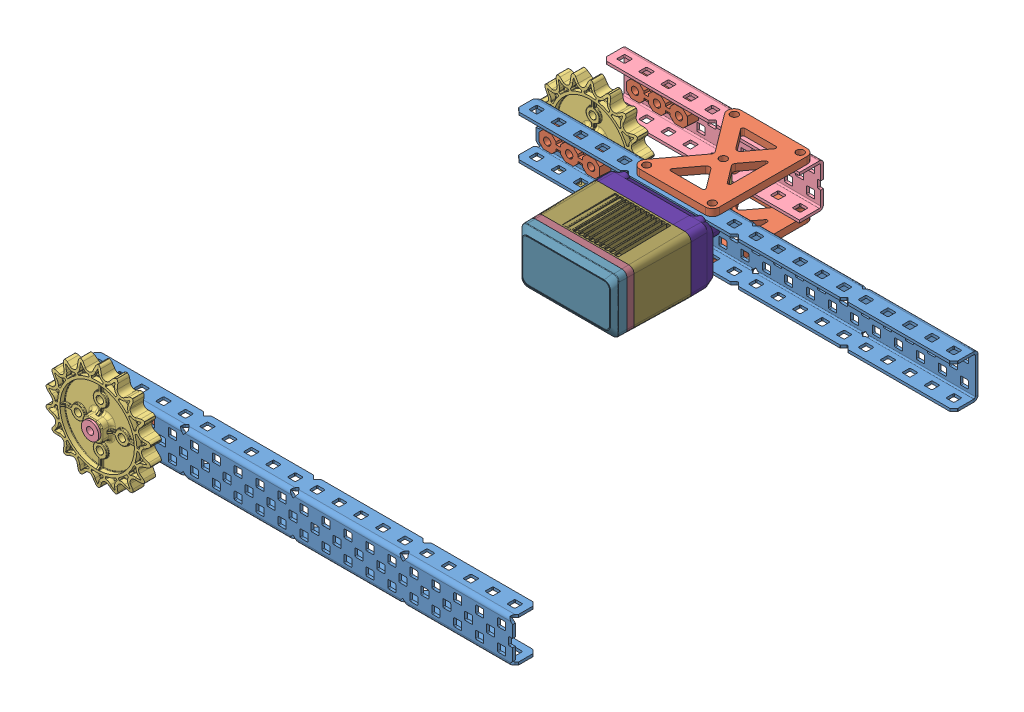
SolidWorks assembly ChainbarTowers, configuration Default. Lengths in mm.
Overall size (259.11 61.52 335.92).
45 component instances, 22 part files, 36 mates.
Components (placement in the parent):
- 1x2x1x20 Aluminum C-Channel-1: 1x2x1x20 Aluminum C-Channel [Default] at (148.2233 92.4309 194.0391) size (254 25.41 13.97)
- 1x2x1x20 Aluminum C-Channel-2: 1x2x1x20 Aluminum C-Channel [Default] at (-42.2767 92.4309 -75.2009) x (-1 0 0) z (0 0 -1) size (254 25.41 13.97)
- Flat Bearing (276-1209)-1: Flat Bearing (276-1209) [Default] at (-22.2107 79.7309 103.4881) x (0 0 1) z (0 -1 0) size (7.04 35.56 10.16)
- Flat Bearing (276-1209)-2: Flat Bearing (276-1209) [Default] at (-75.0427 79.7309 15.3501) x (0 0 -1) z (0 -1 0) size (7.04 35.56 10.16)
- 18THS_Sprocket_w_Inserts-1: 18THS_Sprocket_w_Inserts [Default] at (-67.509 55.75 -129.4065) size (61.01 61.52 15.88)
  - 18T High Strength Sprocket (HS Bore) (276-3878)-1: 18T High Strength Sprocket (HS Bore) (276-3878) [Default] at (18.8823 36.6809 46.2681) size (61.01 61.52 13.34)
  - Plastic Shaft Inserts (276-3881-001)-1: Plastic Shaft Inserts (276-3881-001) [Default] at (18.8823 36.6809 54.2056) x (1 0 0) z (0 1 0) size (10.03 5.08 10.03)
  - Plastic Shaft Inserts (276-3881-001)-2: Plastic Shaft Inserts (276-3881-001) [Default] at (18.8823 36.6809 38.3306) x (0 -1 0) z (-1 0 0) size (10.03 5.08 10.03)
- 18THS_Sprocket_w_Inserts-2: 18THS_Sprocket_w_Inserts [Default] at (-67.509 55.75 155.7085) size (61.01 61.52 15.88)
  - 18T High Strength Sprocket (HS Bore) (276-3878)-1: 18T High Strength Sprocket (HS Bore) (276-3878) [Default] at (18.8823 36.6809 46.2681) size (61.01 61.52 13.34)
  - Plastic Shaft Inserts (276-3881-001)-1: Plastic Shaft Inserts (276-3881-001) [Default] at (18.8823 36.6809 54.2056) x (1 0 0) z (0 1 0) size (10.03 5.08 10.03)
  - Plastic Shaft Inserts (276-3881-001)-2: Plastic Shaft Inserts (276-3881-001) [Default] at (18.8823 36.6809 38.3306) x (0 -1 0) z (-1 0 0) size (10.03 5.08 10.03)
- Flat Bearing (276-1209)-3: Flat Bearing (276-1209) [Default] at (28.5893 79.7309 -164.1771) x (0 0 1) z (0 -1 0) size (7.04 35.56 10.16)
- V5 Smart Motor (276-4840) 2-1: V5 Smart Motor (276-4840) 2 [Default] at (14.8733 92.4309 -29.4261) x (-1 0 0) z (0 0 -1) size (59.01 35.33 72.31)
  - V5 Smart Motor (276-4840) 2.step-1: V5 Smart Motor (276-4840) 2.step [Default] at origin size (59.01 35.33 72.31)
    - 276-4840-900 Rev6_Instruction.step-1: 276-4840-900 Rev6_Instruction.step [Default] at (-14.3 0 -17.2) size (52.79 15.94 38.15)
      - 276-4840-901 Rev6.step-1: 276-4840-901 Rev6.step [Default] at (10.75 -10.05 17.8) x (-1 0 0) z (0 0 1) size (49.9 1.6 38.15)
      - 276-4840-902 Rev2.step-1: 276-4840-902 Rev2.step [Default] at (31.25 -9.25 6.2) x (0 0 -1) z (0 -1 0) size (10.35 11.39 15.94)
      - 276-4840-022 Rev4.step-1: 276-4840-022 Rev4.step [Default] at (31.25 -9.25 6.2) x (0 0 -1) z (1 0 0) size (10.26 9.1 5.51)
    - 276-4840-110 Rev10_Instruction.step-1: 276-4840-110 Rev10_Instruction.step [Default] at (12.7 0 14.7) size (35.33 35.33 31.1)
      - 276-4840-061 Rev7_Ring_Gear_Fixed01 .6 Rev3.step-1: 276-4840-061 Rev7_Ring_Gear_Fixed01 .6 Rev3.step [Default] at origin size (28.79 28.39 24.6)
      - 276-4840-018 Rev6.step-1: 276-4840-018 Rev6.step [Default] at (0 0 6.7) x (-0.483174 0.875524 0) z (0 0 1) size (26 26 12.3)
      - 276-4840-059 Rev2.step-1: 276-4840-059 Rev2.step [Default] at (0 0 10.3) size (28.4 28.4 8.5)
      - 276-4840-062 Rev1.step-1: 276-4840-062 Rev1.step [Default] at (-12.1353 8.8168 12.3) x (0.956835 -0.290632 0) z (-0.290632 -0.956835 0) size (3.2 6.56 3.2)
      - 276-4840-062 Rev1.step-2: 276-4840-062 Rev1.step [Default] at (12.1353 8.8168 12.3) x (0.978427 0.206591 0) z (0.206591 -0.978427 0) size (3.2 6.56 3.2)
      - 276-4840-062 Rev1.step-3: 276-4840-062 Rev1.step [Default] at (-12.1353 -8.8168 12.3) x (0.72563 0.688086 0) z (0.688086 -0.72563 0) size (3.2 6.56 3.2)
    - 276-4840-001 Rev38.step-1: 276-4840-001 Rev38.step [Default] at origin size (57.3 33 46.9)
    - 276-4840-005 Rev27.step-1: 276-4840-005 Rev27.step [Default] at (0 0 -17.95) size (56.17 31.87 12.9)
    - 276-4840-004 Rev16.step-1: 276-4840-004 Rev16.step [Default] at (0 0 -19.2) size (56.01 31.71 9.21)
    - 276-4840-015 Rev7.step-1: 276-4840-015 Rev7.step [Default] at (-21.95 14 27.9) x (-0.85131 -0.524663 0) z (-0.524663 0.85131 0) size (3.2 17.55 3.2)
    - 276-4840-015 Rev7.step-2: 276-4840-015 Rev7.step [Default] at (21.95 -14 27.9) x (-0.777574 -0.628792 0) z (-0.628792 0.777574 0) size (3.2 17.55 3.2)
    - 276-4840-015 Rev7.step-3: 276-4840-015 Rev7.step [Default] at (21.95 14 27.9) x (0.476859 0.87898 0) z (0.87898 -0.476859 0) size (3.2 17.55 3.2)
    - 276-4840-009 Rev3.step-1: 276-4840-009 Rev3.step [Default] at (25.45 13.5 15.7) x (0.19987 -0.979823 0) z (-0.979823 -0.19987 0) size (3.4 41.31 4.34)
    - 276-4840-009 Rev3.step-2: 276-4840-009 Rev3.step [Default] at (-25.45 -13.5 15.7) x (-0.998855 0.047836 0) z (0.047836 0.998855 0) size (3.4 41.31 4.34)
    - 276-4840-009 Rev3.step-3: 276-4840-009 Rev3.step [Default] at (25.45 -13.5 15.7) x (-0.975374 0.220559 0) z (0.220559 0.975374 0) size (3.4 41.31 4.34)
    - 276-4840-009 Rev3.step-4: 276-4840-009 Rev3.step [Default] at (-25.45 13.5 15.7) x (-0.922256 0.38658 0) z (0.38658 0.922256 0) size (3.4 41.31 4.34)
    - 276-4840-003 Rev27.step-1: 276-4840-003 Rev27.step [Default] at (0 0 16.2) size (57.3 33 28.01)
    - 276-4840-043 Rev8.step-1: 276-4840-043 Rev8.step [Default] at (-12.7 0 36.2) x (-0.5 -0.866025 0) z (-0.866025 0.5 0) size (6.3 15.2 7.21)
    - 276-4840-043 Rev8.step-2: 276-4840-043 Rev8.step [Default] at (0 0 36.2) x (-0.5 -0.866025 0) z (-0.866025 0.5 0) size (6.3 15.2 7.21)
    - 276-4840-025 Rev19.step-1: 276-4840-025 Rev19.step [Default] at (12.7 0 -22.63) x (-0.993315 0.115437 0) z (0 0 1) size (14.82 14.83 35.18)
- supportConnector-1: supportConnector [Default] at (33.9233 105.1309 -67.5809) x (0 0 -1) z (0 1 0) size (58.8 46.1 4)
- supportConnector-2: supportConnector [Default] at (33.9233 79.7309 -118.3809) x (0 0 1) z (0 -1 0) size (58.8 46.1 4)
- 1.00_ Standoff (275-1016)-1: 1.00_ Standoff (275-1016) [Default] at (14.8733 92.4309 -92.9809) size (7.34 25.4 7.34)
- 1x2x1x9 Aluminum C-Channel-1: 1x2x1x9 Aluminum C-Channel [Default] at (148.2233 92.4309 -126.0009) x (1 0 0) z (0 0 -1) size (113.79 25.41 13.97)
- Flat Bearing (276-1209)-4: Flat Bearing (276-1209) [Default] at (-22.2107 105.1309 -35.4499) x (0 0 -1) z (0 1 0) size (7.04 35.56 10.16)
Mates (geometry in assembly coordinates):
- Coincident1: coincident aligned: plane of 1x2x1x20 Aluminum C-Channel-1 through (-73.5267 105.1309 226.3978) normal (0 1 0); plane of 1x2x1x20 Aluminum C-Channel-2 through (179.4733 105.1309 -107.5596) normal (0 1 0)
- Parallel1: parallel anti-aligned: plane of 1x2x1x20 Aluminum C-Channel-1 through (-73.5267 70.5106 192.4643) normal (0 0 -1); plane of 1x2x1x20 Aluminum C-Channel-2 through (179.4733 70.5106 -73.6261) normal (0 0 1)
- Distance1: distance = 254 mm: point of 1x2x1x20 Aluminum C-Channel-2; point of 1x2x1x20 Aluminum C-Channel-1
- Concentric1: concentric aligned: circle of 1x2x1x20 Aluminum C-Channel-2; cylinder of Flat Bearing (276-1209)-2 through (-61.3267 92.4309 -67.2761) axis (0 0 -1) radius 2.1209
- Concentric2: concentric aligned: circle of 1x2x1x20 Aluminum C-Channel-2; cylinder of Flat Bearing (276-1209)-2 through (-35.9267 92.4309 -67.2761) axis (0 0 -1) radius 2.1209
- Coincident2: coincident anti-aligned: plane of 1x2x1x20 Aluminum C-Channel-2 through (179.4733 70.5106 -73.6261) normal (0 0 1); plane of Flat Bearing (276-1209)-2 through (-30.843 97.5146 -73.6261) normal (0 0 -1)
- Coincident3: coincident anti-aligned: plane of 1x2x1x20 Aluminum C-Channel-1 through (-73.5267 70.5106 192.4643) normal (0 0 -1); plane of Flat Bearing (276-1209)-1 through (-66.4104 97.5146 192.4643) normal (0 0 1)
- Concentric3: concentric aligned: circle of 1x2x1x20 Aluminum C-Channel-1; cylinder of Flat Bearing (276-1209)-1 through (-61.3267 92.4309 186.1143) axis (0 0 1) radius 2.1209
- Concentric4: concentric aligned: circle of 1x2x1x20 Aluminum C-Channel-1; cylinder of Flat Bearing (276-1209)-1 through (-35.9267 92.4309 186.1143) axis (0 0 1) radius 2.1209
- Concentric5: concentric aligned: cylinder of Flat Bearing (276-1209)-1 through (-61.3267 92.4309 186.1143) axis (0 0 1) radius 2.1209; cylinder of 18THS_Sprocket_w_Inserts-2/18T High Strength Sprocket (HS Bore) (276-3878)-1 through (-61.3267 92.4309 195.3091) axis (0 0 1) radius 2.1
- Concentric6: concentric aligned: cylinder of Flat Bearing (276-1209)-1 through (-35.9267 92.4309 186.1143) axis (0 0 1) radius 2.1209; cylinder of 18THS_Sprocket_w_Inserts-2/18T High Strength Sprocket (HS Bore) (276-3878)-1 through (-35.9267 92.4309 195.3091) axis (0 0 1) radius 2.1
- Coincident4: coincident anti-aligned: plane of 1x2x1x20 Aluminum C-Channel-1 through (-73.5267 70.5106 194.0391) normal (0 0 1); plane of 18THS_Sprocket_w_Inserts-2/Plastic Shaft Inserts (276-3881-001)-2 through (-48.6267 92.4309 194.0391) normal (0 0 -1)
- Concentric7: concentric anti-aligned: cylinder of Flat Bearing (276-1209)-2 through (-61.3267 92.4309 -67.2761) axis (0 0 -1) radius 2.1209; cylinder of 18THS_Sprocket_w_Inserts-1/18T High Strength Sprocket (HS Bore) (276-3878)-1 through (-61.3267 92.4309 -89.8059) axis (0 0 1) radius 2.1
- Concentric8: concentric anti-aligned: cylinder of Flat Bearing (276-1209)-2 through (-35.9267 92.4309 -67.2761) axis (0 0 -1) radius 2.1209; cylinder of 18THS_Sprocket_w_Inserts-1/18T High Strength Sprocket (HS Bore) (276-3878)-1 through (-35.9267 92.4309 -89.8059) axis (0 0 1) radius 2.1
- Coincident5: coincident anti-aligned: plane of 1x2x1x20 Aluminum C-Channel-2 through (179.4733 70.5106 -75.2009) normal (0 0 -1); plane of 18THS_Sprocket_w_Inserts-1/Plastic Shaft Inserts (276-3881-001)-1 through (-48.6267 92.4309 -75.2009) normal (0 0 1)
- Concentric9: concentric anti-aligned: cylinder of 18THS_Sprocket_w_Inserts-1/Plastic Shaft Inserts (276-3881-001)-2 through (-48.6267 92.4309 -91.0759) axis (0 0 -1) radius 2.032; cylinder of 18THS_Sprocket_w_Inserts-2/Plastic Shaft Inserts (276-3881-001)-1 through (-48.6267 92.4309 209.9141) axis (0 0 1) radius 2.032
- Coincident6: coincident anti-aligned: plane of 1x2x1x20 Aluminum C-Channel-2 through (179.4733 70.5106 -73.6261) normal (0 0 1); plane of V5 Smart Motor (276-4840) 2-1/V5 Smart Motor (276-4840) 2.step-1/276-4840-003 Rev27.step-1 through (27.5733 92.4309 -73.6261) normal (0 0 -1)
- Concentric10: concentric anti-aligned: circle of 1x2x1x20 Aluminum C-Channel-2; cylinder of Flat Bearing (276-1209)-3 through (-10.5267 92.4309 -81.5509) axis (0 0 1) radius 2.1209
- Parallel2: parallel: plane of 1x2x1x20 Aluminum C-Channel-2 through (179.4733 105.1309 -107.5596) normal (0 1 0); line of Flat Bearing (276-1209)-3 through (-13.0682 97.5109 -75.2009) axis (1 0 0)
- Coincident8: coincident anti-aligned: plane of 1x2x1x20 Aluminum C-Channel-2 through (179.4733 70.5106 -75.2009) normal (0 0 -1); plane of Flat Bearing (276-1209)-3 through (-15.6104 97.5146 -75.2009) normal (0 0 1)
- Concentric11: concentric aligned: circle of V5 Smart Motor (276-4840) 2-1/V5 Smart Motor (276-4840) 2.step-1/276-4840-003 Rev27.step-1; circle of 1x2x1x20 Aluminum C-Channel-2
- Parallel3: parallel: plane of 1x2x1x20 Aluminum C-Channel-2 through (179.4733 105.1309 -107.5596) normal (0 1 0); line of V5 Smart Motor (276-4840) 2-1/V5 Smart Motor (276-4840) 2.step-1/276-4840-003 Rev27.step-1 through (-4.654 106.81 -58.6261) axis (1 0 0)
- Coincident10: coincident anti-aligned: plane of 1x2x1x20 Aluminum C-Channel-2 through (179.4733 105.1309 -107.5596) normal (0 1 0); plane of supportConnector-1 through (33.9233 105.1309 -67.5809) normal (0 -1 0)
- Concentric12: concentric anti-aligned: circle of 1x2x1x20 Aluminum C-Channel-2; cylinder of supportConnector-1 through (-4.1767 109.1309 -67.5809) axis (0 -1 0) radius 2.15
- Concentric14: concentric anti-aligned: circle of 1x2x1x20 Aluminum C-Channel-2; cylinder of supportConnector-1 through (33.9233 109.1309 -67.5809) axis (0 -1 0) radius 2.15
- Coincident11: coincident anti-aligned: plane of 1x2x1x20 Aluminum C-Channel-2 through (179.4733 79.7309 -63.719) normal (0 -1 0); plane of supportConnector-2 through (33.9233 79.7309 -118.3809) normal (0 1 0)
- Concentric15: concentric anti-aligned: cylinder of supportConnector-1 through (33.9233 109.1309 -118.3809) axis (0 -1 0) radius 2.15; cylinder of supportConnector-2 through (33.9233 75.7309 -118.3809) axis (0 1 0) radius 2.15
- Concentric16: concentric anti-aligned: cylinder of supportConnector-1 through (-4.1767 109.1309 -118.3809) axis (0 -1 0) radius 2.15; cylinder of supportConnector-2 through (-4.1767 75.7309 -118.3809) axis (0 1 0) radius 2.15
- Coincident13: coincident anti-aligned: plane of supportConnector-2 through (33.9233 79.7309 -118.3809) normal (0 1 0); plane of 1x2x1x9 Aluminum C-Channel-1 through (-73.5267 79.7309 -158.3596) normal (0 -1 0)
- Concentric18: concentric anti-aligned: cylinder of supportConnector-2 through (33.9233 75.7309 -118.3809) axis (0 1 0) radius 2.15; circle of 1x2x1x9 Aluminum C-Channel-1
- Concentric19: concentric anti-aligned: cylinder of supportConnector-2 through (-4.1767 75.7309 -118.3809) axis (0 1 0) radius 2.15; circle of 1x2x1x9 Aluminum C-Channel-1
- Concentric20: concentric anti-aligned: cylinder of supportConnector-1 through (14.8733 109.1309 -92.9809) axis (0 -1 0) radius 2.15; cylinder of 1.00_ Standoff (275-1016)-1 through (14.8733 79.7309 -92.9809) axis (0 1 0) radius 2.0955
- Coincident14: coincident anti-aligned: plane of supportConnector-1 through (33.9233 105.1309 -67.5809) normal (0 -1 0); plane of 1.00_ Standoff (275-1016)-1 through (13.0402 105.1309 -96.1559) normal (0 1 0)
- Coincident15: coincident anti-aligned: plane of 1x2x1x9 Aluminum C-Channel-1 through (-73.5267 114.3512 -124.4261) normal (0 0 1); plane of Flat Bearing (276-1209)-4 through (-66.4104 87.3473 -124.4261) normal (0 0 -1)
- Concentric21: concentric aligned: circle of 1x2x1x9 Aluminum C-Channel-1; cylinder of Flat Bearing (276-1209)-4 through (-61.3267 92.4309 -118.0761) axis (0 0 -1) radius 2.1209
- Parallel4: parallel: plane of 1x2x1x9 Aluminum C-Channel-1 through (-73.5267 79.7309 -158.3596) normal (0 -1 0); line of Flat Bearing (276-1209)-4 through (-63.8682 87.3509 -124.4261) axis (1 0 0)
